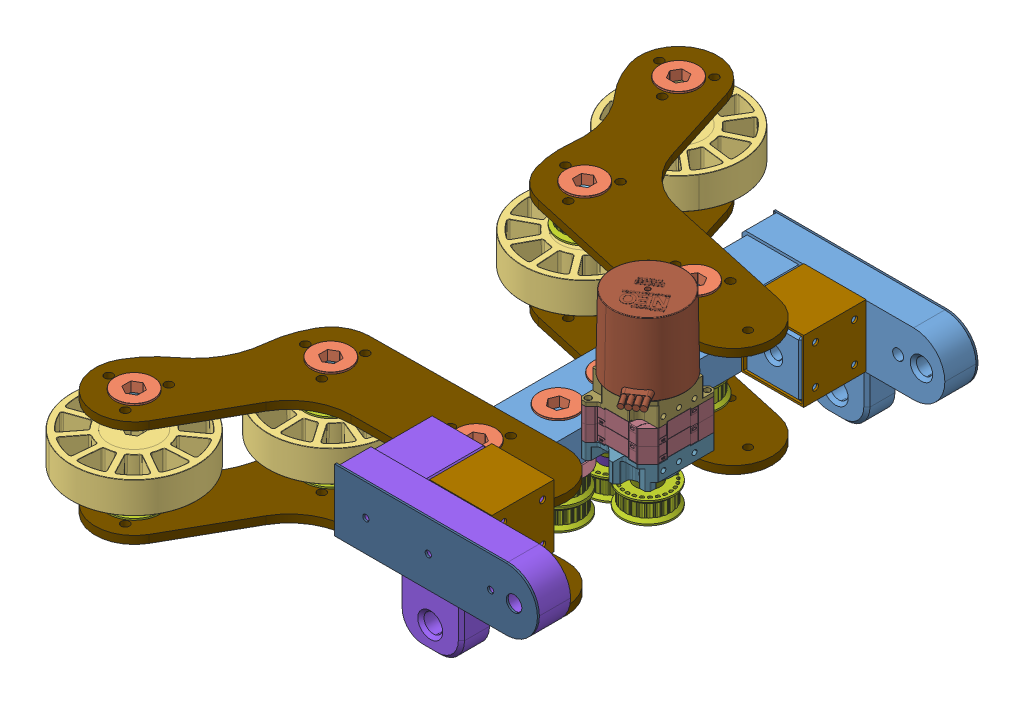
SolidWorks assembly Intake_Claw_2_Wheel_1.0, configuration Default. Lengths in mm. (continued)
Mates (geometry in assembly coordinates): (continued)
- Coincident109: coincident anti-aligned: plane of half_inch_hex_spacer_0.125inch-22 through (-180.9613 -0.381 65.8749) normal (0 -1 0); plane of 24_tooth_5mmHTD_timing_belt_pulley_9mm-20 through (-180.9613 -0.381 65.8749) normal (0 1 0)
- Concentric90: concentric anti-aligned: circle of half_inch_hex_spacer_0.125inch-22; circle of 24_tooth_5mmHTD_timing_belt_pulley_9mm-20
- Coincident110: coincident anti-aligned: plane of half_inch_hex_spacer_0.125inch-31 through (-180.9613 -18.161 65.8749) normal (0 1 0); plane of 24_tooth_5mmHTD_timing_belt_pulley_9mm-20 through (-180.9613 -18.161 65.8749) normal (0 -1 0)
- Concentric91: concentric anti-aligned: circle of half_inch_hex_spacer_0.125inch-31; circle of 24_tooth_5mmHTD_timing_belt_pulley_9mm-20
- Coincident111: coincident anti-aligned: plane of Intake_Plate_Assembly-1/am-2986 FR8ZZ Hex Bearing.step-3 through (-238.9399 -9.4513 -29.6536) normal (0 -1 0); plane of half_inch_hex_spacer_0.125inch-23 through (-150.2116 -14.224 -226.1501) normal (0 1 0)
- Concentric92: concentric anti-aligned: circle of Intake_Plate_Assembly-1/am-2986 FR8ZZ Hex Bearing.step-3; circle of half_inch_hex_spacer_0.125inch-23
- Coincident112: coincident anti-aligned: plane of half_inch_hex_spacer_0.125inch-23 through (-150.2116 -17.399 -226.1501) normal (0 -1 0); plane of 24_tooth_5mmHTD_timing_belt_pulley_9mm-21 through (-150.2116 -17.399 -226.1501) normal (0 1 0)
- Concentric93: concentric anti-aligned: circle of half_inch_hex_spacer_0.125inch-23; circle of 24_tooth_5mmHTD_timing_belt_pulley_9mm-21
- Coincident113: coincident anti-aligned: circle of half_inch_hex_spacer_0.125inch-32; plane of 24_tooth_5mmHTD_timing_belt_pulley_9mm-21 through (-150.2116 -35.179 -226.1501) normal (0 -1 0)
- Concentric94: concentric anti-aligned: circle of half_inch_hex_spacer_0.125inch-32; circle of 24_tooth_5mmHTD_timing_belt_pulley_9mm-21
- Coincident114: coincident anti-aligned: plane of Intake_Plate_Assembly_2-1/am-2986 FR8ZZ Hex Bearing.step-18 through (-242.8184 -9.4513 322.6147) normal (0 -1 0); circle of half_inch_hex_spacer_0.125inch-24
- Concentric95: concentric anti-aligned: circle of Intake_Plate_Assembly_2-1/am-2986 FR8ZZ Hex Bearing.step-18; circle of half_inch_hex_spacer_0.125inch-24
- Coincident115: coincident anti-aligned: plane of half_inch_hex_spacer_0.125inch-24 through (-175.3573 -38.481 192.1035) normal (0 -1 0); plane of 24_tooth_5mmHTD_timing_belt_pulley_9mm-22 through (-175.3573 -38.481 192.1035) normal (0 1 0)
- Concentric96: concentric anti-aligned: circle of half_inch_hex_spacer_0.125inch-24; circle of 24_tooth_5mmHTD_timing_belt_pulley_9mm-22
- Coincident116: coincident anti-aligned: plane of half_inch_hex_spacer_0.125inch-29 through (-175.3573 -56.261 192.1035) normal (0 1 0); plane of 24_tooth_5mmHTD_timing_belt_pulley_9mm-22 through (-175.3573 -56.261 192.1035) normal (0 -1 0)
- Concentric97: concentric anti-aligned: circle of half_inch_hex_spacer_0.125inch-29; circle of 24_tooth_5mmHTD_timing_belt_pulley_9mm-22
- Coincident117: coincident anti-aligned: plane of Intake_Plate_Assembly_2-1/am-2986 FR8ZZ Hex Bearing.step-17 through (-182.211 -9.4513 221.9811) normal (0 -1 0); plane of half_inch_hex_spacer_0.125inch-25 through (-180.9742 2.794 241.8869) normal (0 1 0)
- Concentric98: concentric aligned: circle of Intake_Plate_Assembly_2-1/am-2986 FR8ZZ Hex Bearing.step-17; circle of half_inch_hex_spacer_0.125inch-25
- Coincident120: coincident anti-aligned: plane of Intake_Plate_Assembly_2-1/am-2986 FR8ZZ Hex Bearing.step-11 through (-64.7561 -9.4513 224.1518) normal (0 -1 0); plane of half_inch_hex_spacer_0.125inch-26 through (-117.4709 -35.306 89.8805) normal (0 1 0)
- Concentric101: concentric anti-aligned: circle of Intake_Plate_Assembly_2-1/am-2986 FR8ZZ Hex Bearing.step-11; circle of half_inch_hex_spacer_0.125inch-26
- Coincident121: coincident anti-aligned: plane of half_inch_hex_spacer_0.125inch-26 through (-117.4709 -38.481 89.8805) normal (0 -1 0); plane of 24_tooth_5mmHTD_timing_belt_pulley_9mm-24 through (-117.4709 -38.481 89.8805) normal (0 1 0)
- Concentric102: concentric aligned: circle of Intake_Plate_Assembly_2-1/am-2986 FR8ZZ Hex Bearing.step-11; circle of 24_tooth_5mmHTD_timing_belt_pulley_9mm-24
- Coincident122: coincident anti-aligned: plane of half_inch_hex_spacer_0.125inch-27 through (-117.4709 -56.261 89.8805) normal (0 1 0); plane of 24_tooth_5mmHTD_timing_belt_pulley_9mm-24 through (-117.4709 -56.261 89.8805) normal (0 -1 0)
- Concentric103: concentric anti-aligned: circle of half_inch_hex_spacer_0.125inch-27; circle of 24_tooth_5mmHTD_timing_belt_pulley_9mm-24
- Coincident123: coincident anti-aligned: plane of 24_tooth_5mmHTD_timing_belt_pulley_9mm-18 through (0 -35.179 -88.9) normal (0 -1 0); plane of half_inch_hex_spacer_0.125inch-33 through (0 -35.179 -88.9) normal (0 1 0)
- Concentric104: concentric anti-aligned: circle of 24_tooth_5mmHTD_timing_belt_pulley_9mm-18; circle of half_inch_hex_spacer_0.125inch-33
- Coincident124: coincident anti-aligned: plane of 24_tooth_5mmHTD_timing_belt_pulley_9mm-17 through (0 -35.179 88.9) normal (0 -1 0); plane of half_inch_hex_spacer_0.125inch-34 through (0 -35.179 88.9) normal (0 1 0)
- Concentric105: concentric anti-aligned: circle of 24_tooth_5mmHTD_timing_belt_pulley_9mm-17; circle of half_inch_hex_spacer_0.125inch-34
- Coincident125: coincident anti-aligned: plane of half_inch_hex_spacer_0.125inch-27 through (-117.4709 -59.436 89.8805) normal (0 -1 0); plane of Intake_Plate_Assembly_2-4/am-2986 FR8ZZ Hex Bearing.step-11 through (-63.4848 -33.5813 239.6573) normal (0 1 0)
- Concentric106: concentric aligned: circle of 24_tooth_5mmHTD_timing_belt_pulley_9mm-17; circle of Intake_Plate_Assembly_2-4/am-2986 FR8ZZ Hex Bearing.step-16
- Coincident126: coincident aligned: plane of Intake_Plate_Assembly_2-1/Claw_Intake_Plates-3 through (75.6047 -1.5773 273.9833) normal (-0.018478 0 0.999829); plane of Intake_Plate_Assembly_2-4/Claw_Intake_Plates-3 through (75.6047 -33.6347 273.9833) normal (-0.018478 0 0.999829)
- Coincident127: coincident anti-aligned: plane of half_inch_hex_spacer_0.125inch-33 through (0 -38.354 -88.9) normal (0 -1 0); plane of Intake_Plate_Assembly-3/am-2986 FR8ZZ Hex Bearing.step-5 through (25.4 -33.5813 63.5) normal (0 1 0)
- Concentric107: concentric anti-aligned: circle of half_inch_hex_spacer_0.125inch-33; circle of Intake_Plate_Assembly-3/am-2986 FR8ZZ Hex Bearing.step-5
- Coincident128: coincident aligned: plane of Intake_Plate_Assembly-1/Claw_Intake_Plates-3 through (77.0074 -7.9273 33.08) normal (0.025971 0 -0.999663); plane of Intake_Plate_Assembly-3/Claw_Intake_Plates-3 through (77.0074 -39.9847 33.08) normal (0.025971 0 -0.999663)
- Coincident130: coincident anti-aligned: plane of Intake_Plate_Assembly_2-1/Claw_Intake_Plates-3 through (-241.5471 -1.5773 338.1202) normal (0 1 0); plane of grabber_stand_off-1 through (-122.2369 -23.8023 241.7198) normal (0 -1 0)
- Concentric109: concentric anti-aligned: circle of Claw_Intake_Plates-3; circle of grabber_stand_off-1
- Coincident133: coincident anti-aligned: plane of Intake_Plate_Assembly_2-2/Claw_Intake_Plates-3 through (-236.9809 52.3773 -45.0872) normal (0 -1 0); plane of grabber_stand_off-5 through (-122.2277 50.6322 65.199) normal (0 1 0)
- Concentric111: concentric aligned: circle of Intake_Plate_Assembly_2-2/Claw_Intake_Plates-3; circle of grabber_stand_off-5
- Coincident136: coincident anti-aligned: plane of Claw_Crossbar-1 through (-23.8125 -11.1125 152.4) normal (0 1 0); plane of Grabber_Spring_Mount_2.0-2 through (49.3395 1.5875 0) normal (0 -1 0)
- Coincident137: coincident anti-aligned: plane of Claw_Crossbar-1 through (-23.8125 -11.1125 152.4) normal (0 1 0); plane of Grabber_Spring_Mount_2.0_Right-1 through (23.8125 -11.1125 152.4) normal (0 -1 0)
- Coincident138: coincident anti-aligned: plane of Claw_Crossbar-1 through (23.8125 -11.1125 152.4) normal (-1 0 0); plane of Grabber_Spring_Mount_2.0_Right-1 through (23.8125 35.8775 152.4) normal (1 0 0)
- Coincident139: coincident anti-aligned: plane of Claw_Crossbar-1 through (0 0 152.4) normal (0 0 1); plane of Grabber_Spring_Mount_2.0_Right-1 through (23.8125 35.8775 152.4) normal (0 0 -1)
- Coincident140: coincident aligned: plane of Claw_Crossbar-1 through (-25.4 -12.7 152.4) normal (0 -1 0); plane of Crossbar_Bracket-1 through (76.2 -12.7 -101.6) normal (0 -1 0)
- Coincident141: coincident anti-aligned: plane of Claw_Crossbar-1 through (25.4 -12.7 152.4) normal (1 0 0); plane of Crossbar_Bracket-1 through (25.4 -12.7 -101.6) normal (-1 0 0)
- Coincident142: coincident: line of Claw_Crossbar-1 through (-25.4 -12.7 -152.4) axis (1 0 0); plane of Crossbar_Bracket-1 through (76.2 -12.7 -152.4) normal (0 0 -1)
- Coincident143: coincident anti-aligned: plane of Claw_Crossbar-1 through (25.4 -12.7 152.4) normal (1 0 0); plane of Crossbar_Bracket-2 through (25.4 -12.7 152.4) normal (-1 0 0)
- Coincident144: coincident aligned: plane of Claw_Crossbar-1 through (-25.4 -12.7 152.4) normal (0 -1 0); plane of Crossbar_Bracket-2 through (76.2 -12.7 152.4) normal (0 -1 0)
- Coincident145: coincident: plane of Claw_Crossbar-1; plane of Crossbar_Bracket-2 through (76.2 -12.7 152.4) normal (0 0 1)
- Coincident146: coincident anti-aligned: plane of Grabber_Spring_Mount_2.0_Right-1 through (23.8125 35.8775 177.8) normal (0 0 1); plane of Claw_Pivot_Plate-1 through (114.935 12.065 177.8) normal (0 0 -1)
- Coincident147: coincident anti-aligned: plane of Grabber_Spring_Mount_2.0-2 through (49.3395 1.5875 -25.4) normal (0 0 -1); plane of Claw_Pivot_Plate-2 through (114.935 12.065 -177.8) normal (0 0 1)
- Coincident148: coincident aligned: plane of Grabber_Spring_Mount_2.0-2 through (51.562 0 -25.4) normal (0 -1 0); plane of Claw_Pivot_Plate-2 through (-24.765 -13.335 -177.8) normal (0 -1 0)
- Coincident149: coincident aligned: plane of Grabber_Spring_Mount_2.0_Right-1 through (26.035 -13.335 177.8) normal (0 -1 0); plane of Claw_Pivot_Plate-1 through (-24.765 -13.335 179.3875) normal (0 -1 0)
- Coincident151: coincident anti-aligned: plane of am-2986 FR8ZZ Hex Bearing.step-19 through (-5.7321 -14.224 103.363) normal (0 -1 0); plane of half_inch_hex_spacer_0.125inch-20 through (0 -14.224 88.9) normal (0 1 0)
- Coincident152: coincident anti-aligned: plane of half_inch_hex_spacer_0.125inch-16 through (-117.4709 -35.306 89.8805) normal (0 -1 0); plane of half_inch_hex_spacer_0.125inch-26 through (-117.4709 -35.306 89.8805) normal (0 1 0)
- Coincident153: coincident anti-aligned: plane of half_inch_hex_spacer_0.125inch-17 through (-180.9742 2.794 241.8869) normal (0 -1 0); plane of half_inch_hex_spacer_0.125inch-25 through (-180.9742 2.794 241.8869) normal (0 1 0)
- Coincident154: coincident anti-aligned: plane of am-2986 FR8ZZ Hex Bearing.step-18 through (-5.7321 -14.224 -74.437) normal (0 -1 0); plane of half_inch_hex_spacer_0.125inch-19 through (0 -14.224 -88.9) normal (0 1 0)
- Coincident155: coincident anti-aligned: plane of am-2986 FR8ZZ Hex Bearing.step-16 through (-0.3648 14.224 -104.4532) normal (0 1 0); plane of half_inch_hex_spacer_0.1875inch-1 through (0 14.224 -88.9) normal (0 -1 0)
- Coincident157: coincident anti-aligned: plane of am-2986 FR8ZZ Hex Bearing.step-11 through (-117.4709 14.224 89.8805) normal (0 -1 0); plane of half_inch_hex_spacer_0.125inch-35 through (-117.4709 14.224 89.8805) normal (0 1 0)
- Concentric117: concentric anti-aligned: circle of am-3480 4IN 500Hex Bore Compliant Wheel REV2.STEP-3; circle of half_inch_hex_spacer_0.125inch-35
- Coincident158: coincident aligned: circle of 24_tooth_5mmHTD_timing_belt_pulley_9mm-15; plane of half_inch_hex_spacer_0.125inch-35 through (-117.4709 11.049 89.8805) normal (0 -1 0)
- Concentric118: concentric anti-aligned: circle of 24_tooth_5mmHTD_timing_belt_pulley_9mm-3; circle of half_inch_hex_spacer_0.125inch-36
- Coincident160: coincident anti-aligned: plane of am-2986 FR8ZZ Hex Bearing.step-3 through (-175.3573 14.224 192.1035) normal (0 -1 0); plane of half_inch_hex_spacer_0.125inch-37 through (-175.3573 14.224 192.1035) normal (0 1 0)
- Concentric119: concentric aligned: circle of half_inch_hex_spacer_0.125inch-24; circle of half_inch_hex_spacer_0.125inch-37
- Coincident162: coincident anti-aligned: plane of half_inch_hex_spacer_0.125inch-18 through (-175.3573 -35.306 192.1035) normal (0 -1 0); plane of half_inch_hex_spacer_0.125inch-24 through (-175.3573 -35.306 192.1035) normal (0 1 0)
- Coincident163: coincident aligned: circle of 24_tooth_5mmHTD_timing_belt_pulley_9mm-13; plane of half_inch_hex_spacer_0.125inch-39 through (-180.9613 49.149 65.8749) normal (0 -1 0)
- Concentric120: concentric anti-aligned: circle of 24_tooth_5mmHTD_timing_belt_pulley_9mm-13; circle of half_inch_hex_spacer_0.125inch-39
- Coincident164: coincident aligned: circle of 24_tooth_5mmHTD_timing_belt_pulley_9mm-16; plane of half_inch_hex_spacer_0.125inch-38 through (-114.7265 32.131 -114.1627) normal (0 -1 0)
- Concentric121: concentric anti-aligned: circle of 24_tooth_5mmHTD_timing_belt_pulley_9mm-16; circle of half_inch_hex_spacer_0.125inch-38
- Coincident167: coincident anti-aligned: plane of half_inch_hex_spacer_0.125inch-14 through (-180.9613 2.794 65.8749) normal (0 -1 0); plane of half_inch_hex_spacer_0.125inch-22 through (-180.9613 2.794 65.8749) normal (0 1 0)
- Concentric122: concentric aligned: circle of Claw_Intake_Plates-4; circle of am-2986 FR8ZZ Hex Bearing.step-20
- Coincident168: coincident anti-aligned: plane of Claw_Intake_Plates-4 through (-239.4221 -27.7393 343.7898) normal (0 -1 0); plane of am-2986 FR8ZZ Hex Bearing.step-20 through (13.97 -65.8393 88.9) normal (0 1 0)
- Coincident169: coincident anti-aligned: plane of Claw_Intake_Plates-4 through (-239.4221 -27.7393 343.7898) normal (0 -1 0); plane of am-2986 FR8ZZ Hex Bearing.step-21 through (-106.0114 -27.7393 81.8904) normal (0 1 0)
- Coincident170: coincident anti-aligned: plane of Claw_Intake_Plates-4 through (-239.4221 -27.7393 343.7898) normal (0 -1 0); plane of am-2986 FR8ZZ Hex Bearing.step-22 through (-167.0042 -27.7393 241.8869) normal (0 1 0)
- Concentric123: concentric aligned: circle of Claw_Intake_Plates-4; circle of am-2986 FR8ZZ Hex Bearing.step-22
- Coincident171: coincident anti-aligned: plane of Claw_Intake_Plates-4 through (-239.4221 -27.7393 343.7898) normal (0 -1 0); plane of am-2986 FR8ZZ Hex Bearing.step-23 through (-161.3873 -65.8393 192.1035) normal (0 1 0)
- Concentric124: concentric anti-aligned: cone of Claw_Intake_Plates-4; cylinder of am-2986 FR8ZZ Hex Bearing.step-23 through (-175.3573 -67.2363 192.1035) axis (0 -1 0) radius 785.3982
- Coincident173: coincident aligned: plane of Claw_Intake_Plates-3 through (76.2901 58.7273 272.9054) normal (0.002844 0 0.999996); plane of Claw_Intake_Plates-4 through (76.2901 -21.3893 272.9054) normal (0.002844 0 0.999996)
- Coincident174: coincident anti-aligned: plane of half_inch_hex_spacer_0.125inch-29 through (-175.3573 -59.436 192.1035) normal (0 -1 0); plane of am-2986 FR8ZZ Hex Bearing.step-23 through (-175.3573 -59.436 192.1035) normal (0 1 0)
- Concentric125: concentric anti-aligned: circle of half_inch_hex_spacer_0.125inch-20; circle of am-2986 FR8ZZ Hex Bearing.step-20
- Concentric126: concentric aligned: circle of am-2986 FR8ZZ Hex Bearing.step-19; circle of 24_tooth_5mmHTD_timing_belt_pulley_9mm-17
- Coincident175: coincident anti-aligned: plane of Claw_Intake_Plates-6 through (-240.8657 -32.0573 -35.1788) normal (0 -1 0); plane of am-2986 FR8ZZ Hex Bearing.step-24 through (13.97 -44.7573 -88.9) normal (0 1 0)
- Concentric127: concentric anti-aligned: circle of Claw_Intake_Plates-6; circle of am-2986 FR8ZZ Hex Bearing.step-24
- Coincident176: coincident anti-aligned: circle of Claw_Intake_Plates-6; plane of am-2986 FR8ZZ Hex Bearing.step-25 through (-100.7565 -44.7573 -114.1627) normal (0 1 0)
- Concentric128: concentric aligned: circle of Claw_Intake_Plates-6; circle of am-2986 FR8ZZ Hex Bearing.step-25
- Coincident177: coincident anti-aligned: plane of Claw_Intake_Plates-6 through (-240.8657 -32.0573 -35.1788) normal (0 -1 0); plane of am-2986 FR8ZZ Hex Bearing.step-27 through (-166.9913 -32.0573 65.8749) normal (0 1 0)
- Concentric129: concentric aligned: circle of Claw_Intake_Plates-6; circle of am-2986 FR8ZZ Hex Bearing.step-27
- Coincident178: coincident anti-aligned: plane of Claw_Intake_Plates-6 through (-240.8657 -32.0573 -35.1788) normal (0 -1 0); plane of am-2986 FR8ZZ Hex Bearing.step-26 through (-149.3738 -44.7573 -240.095) normal (0 1 0)
- Concentric130: concentric anti-aligned: circle of Claw_Intake_Plates-6; circle of am-2986 FR8ZZ Hex Bearing.step-26
- Coincident179: coincident anti-aligned: plane of Claw_Intake_Plates-5 through (-240.8657 58.7273 -35.1788) normal (0 1 0); plane of am-2986 FR8ZZ Hex Bearing.step-28 through (13.97 44.1427 -88.9) normal (0 -1 0)
- Concentric131: concentric anti-aligned: circle of Claw_Intake_Plates-5; circle of am-2986 FR8ZZ Hex Bearing.step-28
- Coincident180: coincident anti-aligned: plane of Claw_Intake_Plates-5 through (-240.8657 58.7273 -35.1788) normal (0 1 0); plane of am-2986 FR8ZZ Hex Bearing.step-29 through (-49.5241 58.7273 64.523) normal (0 -1 0)
- Concentric132: concentric aligned: circle of Claw_Intake_Plates-5; circle of am-2986 FR8ZZ Hex Bearing.step-29
- Coincident181: coincident anti-aligned: plane of Claw_Intake_Plates-5 through (-240.8657 58.7273 -35.1788) normal (0 1 0); plane of am-2986 FR8ZZ Hex Bearing.step-30 through (-166.9913 58.7273 65.8749) normal (0 -1 0)
- Concentric133: concentric aligned: circle of Claw_Intake_Plates-5; circle of am-2986 FR8ZZ Hex Bearing.step-30
- Coincident182: coincident anti-aligned: plane of Claw_Intake_Plates-5 through (-240.8657 58.7273 -35.1788) normal (0 1 0); plane of am-2986 FR8ZZ Hex Bearing.step-31 through (-136.2416 44.1427 -226.1501) normal (0 -1 0)
- Concentric134: concentric anti-aligned: circle of Claw_Intake_Plates-5; circle of am-2986 FR8ZZ Hex Bearing.step-31
- Coincident183: coincident anti-aligned: plane of half_inch_hex_spacer_0.125inch-39 through (-180.9613 52.324 65.8749) normal (0 1 0); plane of am-2986 FR8ZZ Hex Bearing.step-30 through (-180.9613 52.324 65.8749) normal (0 -1 0)
- Concentric135: concentric aligned: circle of half_inch_hex_spacer_0.1875inch-1; circle of am-2986 FR8ZZ Hex Bearing.step-28
- Concentric136: concentric anti-aligned: circle of am-2986 FR8ZZ Hex Bearing.step-16; circle of am-2986 FR8ZZ Hex Bearing.step-28
- Coincident184: coincident anti-aligned: plane of half_inch_hex_spacer_0.125inch-33 through (0 -38.354 -88.9) normal (0 -1 0); plane of am-2986 FR8ZZ Hex Bearing.step-24 through (0 -38.354 -88.9) normal (0 1 0)
- Concentric137: concentric aligned: circle of half_inch_hex_spacer_0.125inch-33; circle of am-2986 FR8ZZ Hex Bearing.step-24
- Concentric138: concentric aligned: circle of am-2986 FR8ZZ Hex Bearing.step-18; circle of half_inch_hex_spacer_0.125inch-19
- Coincident185: coincident aligned: plane of Claw_Intake_Plates-5 through (75.8313 52.3773 31.1675) normal (-0.011508 0 -0.999934); plane of Claw_Intake_Plates-6 through (75.8313 -32.0573 31.1675) normal (-0.011508 0 -0.999934)
- Concentric139: concentric anti-aligned: circle of am-3480 4IN 500Hex Bore Compliant Wheel REV2.STEP-3; circle of am-2986 FR8ZZ Hex Bearing.step-21
- Concentric142: concentric anti-aligned: circle of Claw_Intake_Plates-4; circle of am-2986 FR8ZZ Hex Bearing.step-21
- Concentric143: concentric aligned: circle of half_inch_hex_spacer_0.125inch-16; circle of half_inch_hex_spacer_0.125inch-27
- Concentric144: concentric aligned: circle of half_inch_hex_spacer_0.125inch-16; circle of half_inch_hex_spacer_0.125inch-26
- Concentric145: concentric aligned: circle of half_inch_hex_spacer_0.125inch-28; circle of am-2986 FR8ZZ Hex Bearing.step-22
- Coincident190: coincident aligned: circle of half_inch_hex_spacer_0.125inch-17; circle of half_inch_hex_spacer_0.125inch-25
- Concentric146: concentric aligned: circle of half_inch_hex_spacer_0.125inch-29; circle of am-2986 FR8ZZ Hex Bearing.step-23
- Coincident191: coincident aligned: circle of half_inch_hex_spacer_0.125inch-18; circle of half_inch_hex_spacer_0.125inch-24
- Concentric147: concentric anti-aligned: circle of half_inch_hex_spacer_0.125inch-30; circle of am-2986 FR8ZZ Hex Bearing.step-25
- Concentric149: concentric aligned: circle of am-3480 4IN 500Hex Bore Compliant Wheel REV2.STEP-4; circle of am-2986 FR8ZZ Hex Bearing.step-25
- Concentric150: concentric anti-aligned: circle of half_inch_hex_spacer_0.125inch-38; circle of am-2986 FR8ZZ Hex Bearing.step-29
- Concentric151: concentric anti-aligned: circle of half_inch_hex_spacer_0.125inch-39; circle of am-2986 FR8ZZ Hex Bearing.step-30
- Concentric152: concentric anti-aligned: circle of half_inch_hex_spacer_0.125inch-31; circle of am-2986 FR8ZZ Hex Bearing.step-27
- Concentric153: concentric anti-aligned: circle of half_inch_hex_spacer_0.125inch-14; circle of am-2986 FR8ZZ Hex Bearing.step-27
- Concentric154: concentric aligned: circle of grabber_stand_off-5; circle of Claw_Intake_Plates-6
- Concentric156: concentric anti-aligned: circle of half_inch_hex_spacer_0.125inch-32; circle of am-2986 FR8ZZ Hex Bearing.step-26
- Coincident192: coincident anti-aligned: plane of am-2986 FR8ZZ Hex Bearing.step-13 through (-5.7321 -14.224 -7.762) normal (0 -1 0); plane of half_inch_hex_spacer_0.125inch-1 through (0 -14.224 -22.225) normal (0 1 0)
- Coincident193: coincident anti-aligned: plane of Claw_Drive_Gear-1 through (0 -17.399 -22.225) normal (0 1 0); plane of half_inch_hex_spacer_0.125inch-1 through (0 -17.399 -22.225) normal (0 -1 0)
- Concentric158: concentric aligned: circle of Claw_Crossbar-1; circle of am-2986 FR8ZZ Hex Bearing.step-32
- Coincident195: coincident anti-aligned: plane of Claw_Crossbar-1 through (-25.4 -12.7 152.4) normal (0 -1 0); plane of am-2986 FR8ZZ Hex Bearing.step-32 through (-6.9887 -12.7 34.3212) normal (0 1 0)
- Coincident196: coincident anti-aligned: plane of half_inch_hex_spacer_0.125inch-2 through (0 -14.224 22.225) normal (0 1 0); plane of am-2986 FR8ZZ Hex Bearing.step-32 through (-7.7829 -14.224 35.6958) normal (0 -1 0)
- Coincident197: coincident anti-aligned: plane of Claw_Drive_Gear-2 through (0 -17.399 22.225) normal (0 1 0); plane of half_inch_hex_spacer_0.125inch-2 through (0 -17.399 22.225) normal (0 -1 0)
- Coincident202: coincident anti-aligned: circle of Claw_Drive_Gear-2; plane of half_inch_hex_spacer_0.125inch-2 through (0 -17.399 22.225) normal (0 -1 0)
- Concentric160: concentric aligned: circle of Claw_Drive_Gear-2; circle of half_inch_hex_spacer_0.125inch-2
- Concentric161: concentric anti-aligned: circle of half_inch_hex_spacer_0.125inch-2; circle of am-2986 FR8ZZ Hex Bearing.step-32
- Coincident203: coincident anti-aligned: plane of am-2986 FR8ZZ Hex Bearing.step-20 through (15.5575 -67.3633 88.9) normal (0 -1 0); plane of half_inch_hex_spacer_0.125inch-41 through (0 -67.3633 88.9) normal (0 1 0)
- Concentric162: concentric anti-aligned: circle of am-2986 FR8ZZ Hex Bearing.step-20; circle of half_inch_hex_spacer_0.125inch-41
- Coincident204: coincident anti-aligned: plane of am-2986 FR8ZZ Hex Bearing.step-24 through (15.5575 -46.2813 -88.9) normal (0 -1 0); plane of half_inch_hex_spacer_0.125inch-40 through (0 -46.2813 -88.9) normal (0 1 0)
- Concentric163: concentric anti-aligned: circle of am-2986 FR8ZZ Hex Bearing.step-24; circle of half_inch_hex_spacer_0.125inch-40
- Coincident205: coincident aligned: plane of half_inch_hex_spacer_0.125inch-40 through (0 -49.4563 -88.9) normal (0 -1 0); circle of 24_tooth_5mmHTD_timing_belt_pulley_9mm-25
- Concentric164: concentric anti-aligned: circle of half_inch_hex_spacer_0.125inch-40; circle of 24_tooth_5mmHTD_timing_belt_pulley_9mm-25
- Coincident206: coincident aligned: plane of half_inch_hex_spacer_0.125inch-41 through (0 -70.5383 88.9) normal (0 -1 0); circle of 24_tooth_5mmHTD_timing_belt_pulley_9mm-26
- Concentric165: concentric anti-aligned: circle of half_inch_hex_spacer_0.125inch-41; circle of 24_tooth_5mmHTD_timing_belt_pulley_9mm-26
- Coincident207: coincident anti-aligned: plane of Claw_Drive_Gear-1 through (0 -26.8478 -22.225) normal (0 -1 0); plane of half_inch_hex_spacer_0.5inch-1 through (0 -26.8478 -22.225) normal (0 1 0)
- Concentric166: concentric aligned: circle of Claw_Drive_Gear-1; circle of half_inch_hex_spacer_0.5inch-1
- Coincident208: coincident anti-aligned: plane of half_inch_hex_spacer_0.5inch-1 through (0 -39.5478 -22.225) normal (0 -1 0); plane of half_inch_hex_spacer_0.25inch-1 through (0 -39.5478 -22.225) normal (0 1 0)
- Concentric167: concentric aligned: circle of half_inch_hex_spacer_0.5inch-1; circle of half_inch_hex_spacer_0.25inch-1
- Coincident210: coincident aligned: circle of 24_tooth_5mmHTD_timing_belt_pulley_9mm-9; plane of half_inch_hex_spacer_0.25inch-1 through (0 -45.8978 -22.225) normal (0 -1 0)
- Concentric168: concentric anti-aligned: circle of 24_tooth_5mmHTD_timing_belt_pulley_9mm-9; circle of half_inch_hex_spacer_0.25inch-1
- Distance1: distance = 50.8 mm anti-aligned: plane of am-4700_syc Cone-1 through (-192.6779 79.0118 -94.5539) normal (0.17378 -0.984784 0); plane of Claw_Intake_Plates-3 through (-239.4221 58.7273 343.7898) normal (0 1 0)
- Distance2: distance = 73.9164 mm aligned: plane of am-4700_syc Cone-1 through (-192.6779 79.0118 105.4711) normal (0 0 1); plane of Claw_Pivot_Plate-1 through (114.935 12.065 179.3875) normal (0 0 1)
- Coincident218: coincident anti-aligned: plane of am-2986 FR8ZZ Hex Bearing.step-28 through (13.97 44.1427 -88.9) normal (0 -1 0); plane of Claw_Intake_Plate_2_Wheel-3 through (-211.1629 44.1427 -145.221) normal (0 1 0)
- Concentric171: concentric aligned: circle of am-2986 FR8ZZ Hex Bearing.step-28; circle of Claw_Intake_Plate_2_Wheel-3
- Coincident219: coincident anti-aligned: plane of am-2986 FR8ZZ Hex Bearing.step-24 through (13.97 -44.7573 -88.9) normal (0 1 0); plane of Claw_Intake_Plate_2_Wheel-4 through (-211.1629 -44.7573 -145.221) normal (0 -1 0)
- Concentric172: concentric aligned: circle of am-2986 FR8ZZ Hex Bearing.step-24; circle of Claw_Intake_Plate_2_Wheel-4
- Coincident220: coincident aligned: plane of Claw_Intake_Plate_2_Wheel-3 through (-26.3911 37.7927 -62.2007) normal (-0.215048 0 0.976604); plane of Claw_Intake_Plate_2_Wheel-4 through (-26.3911 -44.7573 -62.2007) normal (-0.215048 0 0.976604)
- Coincident221: coincident anti-aligned: plane of am-2986 FR8ZZ Hex Bearing.step-5 through (0 20.6273 74.93) normal (0 -1 0); plane of Claw_Intake_Plate_2_Wheel-2 through (-218.2465 20.6273 100.3151) normal (0 1 0)
- Concentric173: concentric aligned: circle of am-2986 FR8ZZ Hex Bearing.step-5; circle of Claw_Intake_Plate_2_Wheel-2
- Coincident222: coincident anti-aligned: plane of am-2986 FR8ZZ Hex Bearing.step-20 through (13.97 -65.8393 88.9) normal (0 1 0); plane of Claw_Intake_Plate_2_Wheel-1 through (-218.2465 -65.8393 100.3151) normal (0 -1 0)
- Concentric174: concentric aligned: circle of am-2986 FR8ZZ Hex Bearing.step-20; circle of Claw_Intake_Plate_2_Wheel-1
- Coincident223: coincident aligned: plane of Claw_Intake_Plate_2_Wheel-1 through (41.5386 -59.4893 120.3044) normal (0.008346 0 0.999965); plane of Claw_Intake_Plate_2_Wheel-2 through (41.5386 20.6273 120.3044) normal (0.008346 0 0.999965)
- Concentric175: concentric anti-aligned: circle of am-2986 FR8ZZ Hex Bearing.step-1; circle of am-2986 FR8ZZ Hex Bearing.step-5
- Coincident224: coincident anti-aligned: plane of am-2986 FR8ZZ Hex Bearing.step-23 through (-161.3873 -65.8393 192.1035) normal (0 1 0); plane of Claw_Intake_Plate_2_Wheel-1 through (-218.2465 -65.8393 100.3151) normal (0 -1 0)
- Concentric176: concentric aligned: circle of am-2986 FR8ZZ Hex Bearing.step-23; circle of Claw_Intake_Plate_2_Wheel-1
- Coincident225: coincident anti-aligned: plane of am-2986 FR8ZZ Hex Bearing.step-3 through (-175.3573 20.6273 178.1335) normal (0 -1 0); plane of Claw_Intake_Plate_2_Wheel-2 through (-218.2465 20.6273 100.3151) normal (0 1 0)
- Concentric177: concentric aligned: circle of am-2986 FR8ZZ Hex Bearing.step-3; circle of Claw_Intake_Plate_2_Wheel-2
- Concentric179: concentric aligned: circle of am-2986 FR8ZZ Hex Bearing.step-11; circle of Claw_Intake_Plate_2_Wheel-2
- Concentric180: concentric aligned: circle of am-2986 FR8ZZ Hex Bearing.step-11; circle of am-3480 4IN 500Hex Bore Compliant Wheel REV2.STEP-3
- Coincident229: coincident anti-aligned: plane of am-2986 FR8ZZ Hex Bearing.step-31 through (-136.2416 44.1427 -226.1501) normal (0 -1 0); plane of Claw_Intake_Plate_2_Wheel-3 through (-211.1629 44.1427 -145.221) normal (0 1 0)
- Concentric182: concentric aligned: circle of am-2986 FR8ZZ Hex Bearing.step-31; circle of Claw_Intake_Plate_2_Wheel-3
- Concentric183: concentric anti-aligned: circle of am-3480 4IN 500Hex Bore Compliant Wheel REV2.STEP-6; circle of am-2986 FR8ZZ Hex Bearing.step-31
- Concentric184: concentric anti-aligned: circle of am-2986 FR8ZZ Hex Bearing.step-29; circle of Claw_Intake_Plate_2_Wheel-3
- Concentric185: concentric aligned: circle of am-3480 4IN 500Hex Bore Compliant Wheel REV2.STEP-4; circle of am-2986 FR8ZZ Hex Bearing.step-29
- Concentric186: concentric aligned: circle of am-3480 4IN 500Hex Bore Compliant Wheel REV2.STEP-6; circle of am-2986 FR8ZZ Hex Bearing.step-31
- Coincident231: coincident anti-aligned: plane of am-2986 FR8ZZ Hex Bearing.step-11 through (-117.4709 20.6273 75.9105) normal (0 -1 0); plane of Claw_Intake_Plate_2_Wheel-2 through (-218.2465 20.6273 100.3151) normal (0 1 0)
- Coincident232: coincident anti-aligned: plane of Claw_Intake_Plate_2_Wheel-3 through (-211.1629 44.1427 -145.221) normal (0 1 0); plane of am-2986 FR8ZZ Hex Bearing.step-33 through (-114.7265 44.1427 -128.1327) normal (0 -1 0)
- Concentric187: concentric anti-aligned: circle of Claw_Intake_Plate_2_Wheel-3; circle of am-2986 FR8ZZ Hex Bearing.step-33
- Coincident234: coincident anti-aligned: plane of half_inch_hex_spacer_0.125inch-32 through (-150.2116 -38.354 -226.1501) normal (0 -1 0); plane of am-2986 FR8ZZ Hex Bearing.step-26 through (-150.2116 -38.354 -226.1501) normal (0 1 0)
- Coincident235: coincident anti-aligned: plane of half_inch_hex_spacer_0.125inch-30 through (-114.7265 -38.354 -114.1627) normal (0 -1 0); plane of am-2986 FR8ZZ Hex Bearing.step-25 through (-114.7265 -38.354 -114.1627) normal (0 1 0)
- Coincident236: coincident anti-aligned: plane of am-2986 FR8ZZ Hex Bearing.step-25 through (-100.7565 -44.7573 -114.1627) normal (0 1 0); plane of Claw_Intake_Plate_2_Wheel-4 through (-211.1629 -44.7573 -145.221) normal (0 -1 0)
- Concentric188: concentric aligned: circle of am-2986 FR8ZZ Hex Bearing.step-25; circle of Claw_Intake_Plate_2_Wheel-4
- Concentric189: concentric aligned: circle of half_inch_hex_spacer_0.125inch-38; circle of am-2986 FR8ZZ Hex Bearing.step-33
- Coincident237: coincident anti-aligned: plane of am-2986 FR8ZZ Hex Bearing.step-26 through (-149.3738 -44.7573 -240.095) normal (0 1 0); plane of Claw_Intake_Plate_2_Wheel-4 through (-211.1629 -44.7573 -145.221) normal (0 -1 0)
- Tangent1: tangent anti-aligned: plane of Claw_Crossbar-1 through (-25.4 -12.7 152.4) normal (-1 0 0); cylinder of am-4700_syc Cone-1 through (-99.073 87.5385 -0.8914) axis (0.17378 -0.984784 0) radius 174.6671
- Coincident238: coincident aligned: plane of Claw_Crossbar-1 through (-25.4 -12.7 152.4) normal (0 -1 0); plane of Neo_with_2_Stage_Gearbox-1/REV-21-2104.step-1 through (50.8 -12.7 0) normal (0 -1 0)
- Coincident239: coincident anti-aligned: plane of Claw_Crossbar-1 through (25.4 -12.7 152.4) normal (1 0 0); plane of Neo_with_2_Stage_Gearbox-1/REV-21-2104.step-1 through (25.4 6.35 -25.4) normal (-1 0 0)
- Distance3: distance = 76.2 mm anti-aligned: plane of Neo_with_2_Stage_Gearbox-1/REV-21-2103.step-2 through (25.4 6.35 25.4) normal (0 0 1); plane of Crossbar_Bracket-2 through (76.2 -12.7 101.6) normal (0 0 -1)
- Coincident241: coincident anti-aligned: plane of Claw_Crossbar-1 through (-25.4 12.7 152.4) normal (0 1 0); plane of am-2986 FR8ZZ Hex Bearing.step-34 through (-5.1472 12.7 35.2122) normal (0 -1 0)
- Concentric193: concentric aligned: circle of Claw_Crossbar-1; cylinder of am-2986 FR8ZZ Hex Bearing.step-34 through (0 14.097 22.225) axis (0 1 0) radius 785.3982
- Concentric194: concentric anti-aligned: circle of Claw_Drive_Gear-2; circle of 24_tooth_5mmHTD_timing_belt_pulley_9mm-28
- Coincident243: coincident anti-aligned: plane of Claw_Drive_Gear-2 through (0 -26.8478 22.225) normal (0 -1 0); plane of 24_tooth_5mmHTD_timing_belt_pulley_9mm-28 through (0 -26.8478 22.225) normal (0 1 0)
- Coincident244: coincident aligned: circle of 24_tooth_5mmHTD_timing_belt_pulley_9mm-8; circle of 24_tooth_5mmHTD_timing_belt_pulley_9mm-28
- Concentric195: concentric anti-aligned: circle of Neo_with_2_Stage_Gearbox-1/motor_drive_shaft-1; circle of half_inch_hex_spacer_0.5inch-2
- Coincident245: coincident anti-aligned: plane of Neo_with_2_Stage_Gearbox-1/REV-21-2104.step-1 through (50.8 -12.7 0) normal (0 -1 0); plane of half_inch_hex_spacer_0.5inch-2 through (50.8 -12.7 0) normal (0 1 0)
- Concentric196: concentric anti-aligned: circle of Neo_with_2_Stage_Gearbox-1/motor_drive_shaft-1; cylinder of 24_tooth_5mmHTD_timing_belt_pulley_9mm-27 through (50.8 -43.18 0) axis (0 1 0) radius 21.082
- Coincident246: coincident aligned: circle of half_inch_hex_spacer_0.5inch-2; plane of 24_tooth_5mmHTD_timing_belt_pulley_9mm-27 through (50.8 -25.4 0) normal (0 1 0)
- Distance4: distance = 186.0459 mm: point of Claw_Crossbar-1; moEndPointRef_w of am-4700_syc Cone-1
- Coincident248: coincident anti-aligned: plane of Grabber_Spring_Mount_2.0-2 through (100.0125 48.5775 50.8) normal (1 0 0); plane of Crossbar_Bracket-1 through (74.6125 -11.1125 -101.6) normal (-1 0 0)
- Concentric197: concentric anti-aligned: circle of Grabber_Spring_Mount_2.0-2; circle of Claw_Pivot_Plate-2
- Concentric198: concentric anti-aligned: circle of Grabber_Spring_Mount_2.0-1; circle of Claw_Pivot_Plate-1
- Concentric199: concentric anti-aligned: circle of Grabber_Spring_Mount_2.0_Right-1; circle of Grabber_Spring_Mount_2.0_Left-1
- Coincident250: coincident anti-aligned: plane of Crossbar_Bracket-1 through (76.2 -12.7 -152.4) normal (0 0 -1); plane of Grabber_Spring_Mount_2.0_Left-1 through (23.8125 -11.7475 -152.4) normal (0 0 1)
- Concentric200: concentric aligned: circle of Claw_Pivot_Plate-2; circle of Grabber_Spring_Mount_2.0_Left-1
- Parallel8: parallel aligned: plane of Crossbar_Bracket-1 through (76.2 -12.7 -101.6) normal (0 -1 0); plane of Grabber_Spring_Mount_2.0_Left-1 through (26.035 -13.335 -177.8) normal (0 -1 0)
- Coincident252: coincident anti-aligned: plane of Claw_Pivot_Plate-2 through (114.935 12.065 -177.8) normal (0 0 1); plane of Grabber_Spring_Mount_2.0_Left-1 through (23.8125 -11.7475 -177.8) normal (0 0 -1)
- Coincident253: coincident aligned: plane of Claw_Pivot_Plate-2 through (-24.765 -13.335 -177.8) normal (0 -1 0); plane of Grabber_Spring_Mount_2.0_Left-1 through (26.035 -13.335 -177.8) normal (0 -1 0)
- Coincident254: coincident anti-aligned: plane of am-3480 4IN 500Hex Bore Compliant Wheel REV2.STEP-4 through (-122.9584 -14.224 -99.1232) normal (0 -1 0); plane of half_inch_hex_spacer_0.125inch-21 through (-114.7265 -14.224 -114.1627) normal (0 1 0)
- Coincident255: coincident anti-aligned: plane of am-3480 4IN 500Hex Bore Compliant Wheel REV2.STEP-4 through (-115.9461 11.176 -111.9346) normal (0 1 0); plane of half_inch_hex_spacer_0.125inch-13 through (-114.7265 11.176 -114.1627) normal (0 -1 0)
- Concentric202: concentric aligned: circle of am-3480 4IN 500Hex Bore Compliant Wheel REV2.STEP-4; cylinder of half_inch_hex_spacer_0.125inch-13 through (-114.7265 14.351 -114.1627) axis (0 -1 0) radius 10.16
- Parallel9: parallel aligned: plane of am-3480 4IN 500Hex Bore Compliant Wheel REV2.STEP-4 through (-107.3667 11.176 -114.3305) normal (-0.877194 0 -0.480136); plane of half_inch_hex_spacer_0.125inch-13 through (-110.6118 14.351 -107.3967) normal (-0.877194 0 -0.480136)
- Coincident258: coincident anti-aligned: plane of 24_tooth_5mmHTD_timing_belt_pulley_9mm-16 through (-114.7265 14.351 -114.1627) normal (0 -1 0); plane of half_inch_hex_spacer_0.125inch-13 through (-114.7265 14.351 -114.1627) normal (0 1 0)
- Concentric203: concentric aligned: circle of am-3480 4IN 500Hex Bore Compliant Wheel REV2.STEP-6; cylinder of half_inch_hex_spacer_0.125inch-23 through (-150.2116 -14.224 -226.1501) axis (0 -1 0) radius 10.16
- Coincident259: coincident anti-aligned: plane of am-3480 4IN 500Hex Bore Compliant Wheel REV2.STEP-6 through (-148.8818 -14.224 -228.3142) normal (0 -1 0); circle of half_inch_hex_spacer_0.125inch-23
- Concentric204: concentric aligned: circle of am-3480 4IN 500Hex Bore Compliant Wheel REV2.STEP-6; cylinder of half_inch_hex_spacer_0.125inch-15 through (-150.2116 14.351 -226.1501) axis (0 -1 0) radius 10.16
- Coincident260: coincident anti-aligned: plane of am-3480 4IN 500Hex Bore Compliant Wheel REV2.STEP-6 through (-148.8818 11.176 -228.3142) normal (0 1 0); plane of half_inch_hex_spacer_0.125inch-15 through (-150.2116 11.176 -226.1501) normal (0 -1 0)
